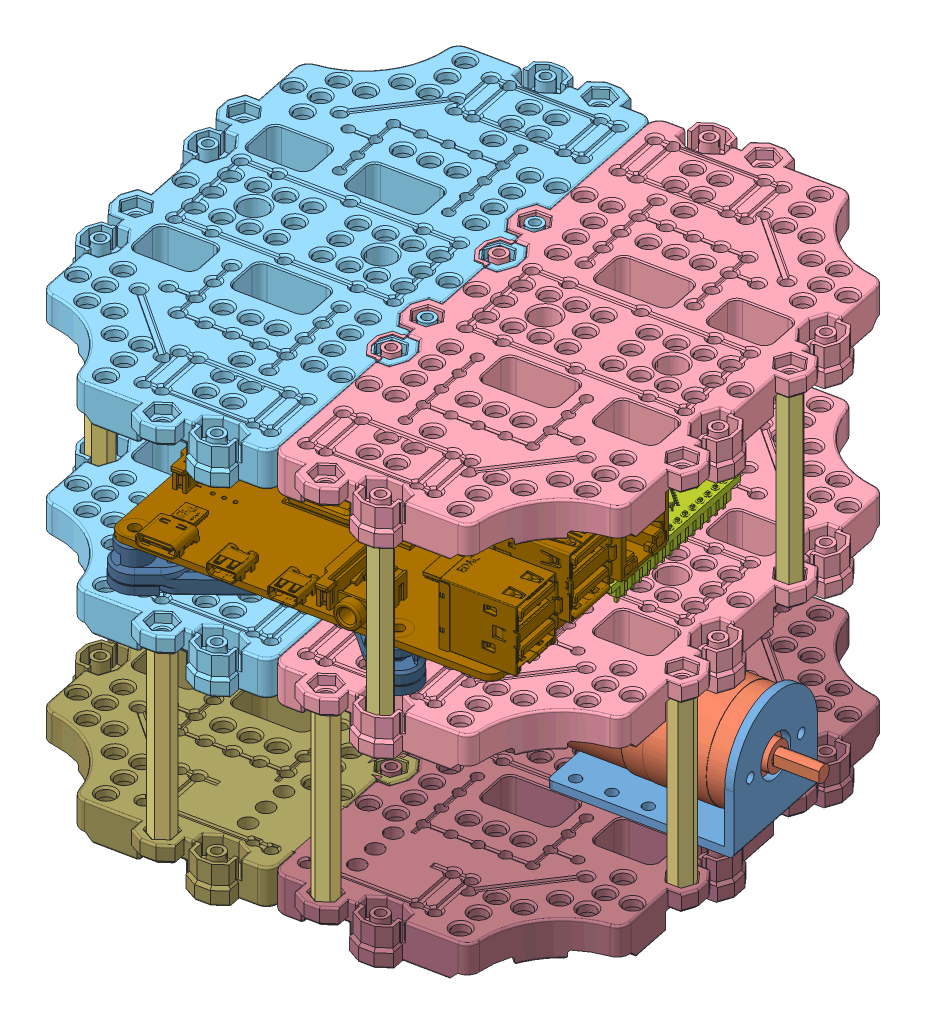
SolidWorks assembly base_link, configuration Default. Lengths in mm.
Overall size (162.47 104.15 162.47).
33 component instances, 13 part files, 91 mates.
Components (placement in the parent):
- motor_support-1: motor_support [Default] at (-43.4369 -3.9762 107.463) x (-0.201684 0 -0.979451) z (0.979451 0 -0.201684) size (28 29 41)
- motor_support-2: motor_support [Default] at (91.2839 -3.9762 79.7219) x (0.201684 0 0.979451) z (-0.979451 0 0.201684) size (28 29 41)
- JGA25-370-1: JGA25-370 [Default] at (46.94 -3.9762 88.853) x (0.979451 0 -0.201684) z (0 -1 0) size (70.5 25.2 25.2)
- JGA25-370-2: JGA25-370 [Default] at (0.907 -3.9762 98.3319) x (-0.979451 0 0.201684) z (0 -1 0) size (70.5 25.2 25.2)
- SUPPORT_HEX_M3_0XL45_FF-1: SUPPORT_HEX_M3_0XL45_FF [Default] at (34.5226 -21.4762 26.0672) x (-0.5 0 0.866025) z (-0.866025 0 -0.5) size (5 45 5.77)
- SUPPORT_HEX_M3_0XL45_FF-6: SUPPORT_HEX_M3_0XL45_FF [Default] at (13.3245 -21.4762 161.1177) x (0.255141 0 -0.966904) z (0.966904 0 0.255141) size (5 45 5.77)
- waffle_front_plate-3: waffle_front_plate [Default] at (23.9235 28.0238 93.5924) x (0.979451 0 -0.201684) z (0.201684 0 0.979451) size (73.55 9.85 137.55)
- waffle_rear_plate-2: waffle_rear_plate [Default] at (23.9235 28.0238 93.5924) x (-0.979451 0 0.201684) z (-0.201684 0 -0.979451) size (73.55 9.85 137.55)
- SUPPORT_HEX_M3_0XL45_FF-7: SUPPORT_HEX_M3_0XL45_FF [Default] at (-12.4911 -23.9762 35.748) x (0 0 -1) z (1 0 0) size (5 45 5.77)
- SUPPORT_HEX_M3_0XL45_FF-17: SUPPORT_HEX_M3_0XL45_FF [Default] at (-43.6018 23.5238 82.9934) x (0.866025 0 0.5) z (0.5 0 -0.866025) size (5 45 5.77)
- SUPPORT_HEX_M3_0XL45_FF-18: SUPPORT_HEX_M3_0XL45_FF [Default] at (91.4488 23.5238 104.1915) x (0.866025 0 0.5) z (0.5 0 -0.866025) size (5 45 5.77)
- L298N-2: L298N [Default] at (1.533 38.0238 65.2768) x (0.979451 0 -0.201684) z (0.201684 0 0.979451) size (50 22 50)
- Arduino Nano-2: Arduino Nano [Default] at (32.4135 30.0238 59.7967) x (0.201684 0 0.979451) z (0 1 0) size (44.28 18 13.68)
- board_bracket_small-1: board_bracket_small [Default] at (19.5539 28.0238 39.0638) x (0.977292 0 -0.211899) z (0.211899 0 0.977292) size (37.82 10 10.43)
- board_bracket_small-2: board_bracket_small [Default] at (-16.4879 28.0238 91.4897) x (0.231228 0 0.9729) z (-0.9729 0 0.231228) size (37.82 10 10.43)
- board_bracket_small-3: board_bracket_small [Default] at (28.444 28.0238 82.2376) x (0.272036 0 0.962287) z (-0.962287 0 0.272036) size (37.82 10 10.43)
- SUPPORT_HEX_M3_0XL45_FF-20: SUPPORT_HEX_M3_0XL45_FF [Default] at (-33.9209 68.3238 130.007) x (0.664389 0 0.747387) z (0.747387 0 -0.664389) size (5 45 5.77)
- SUPPORT_HEX_M3_0XL45_FF-21: SUPPORT_HEX_M3_0XL45_FF [Default] at (-0.7377 70.5238 33.3278) x (-0.979451 0 0.201684) z (0.201684 0 0.979451) size (5 45 5.77)
- SUPPORT_HEX_M3_0XL45_FF-22: SUPPORT_HEX_M3_0XL45_FF [Default] at (-41.1815 68.3238 94.7468) x (-0.315062 0 0.949071) z (0.949071 0 0.315062) size (5 45 5.77)
- SUPPORT_HEX_M3_0XL45_FF-23: SUPPORT_HEX_M3_0XL45_FF [Default] at (22.7691 68.3238 28.4874) x (0.201684 0 0.979451) z (0.979451 0 -0.201684) size (5 45 5.77)
- SUPPORT_HEX_M3_0XL45_FF-25: SUPPORT_HEX_M3_0XL45_FF [Default] at (48.5847 23.5238 153.8571) x (1 0 0) z (0 0 -1) size (5 45 5.77)
- SUPPORT_HEX_M3_0XL45_FF-26: SUPPORT_HEX_M3_0XL45_FF [Default] at (60.3381 68.3238 151.4369) x (0.949071 0 0.315062) z (0.315062 0 -0.949071) size (5 45 5.77)
- SUPPORT_HEX_M3_0XL45_FF-27: SUPPORT_HEX_M3_0XL45_FF [Default] at (84.1881 70.5238 68.9313) x (0.201684 0 0.979451) z (0.979451 0 -0.201684) size (5 45 5.77)
- Raspberry Pi 4 Model B-3: Raspberry Pi 4 Model B [Default] at (147.2874 -46.1762 96.888) x (0.979451 0 -0.201684) z (0 1 0) size (89.07 58.45 20.84)
- board_bracket-5: board_bracket [Default] at (57.1744 28.0238 143.6412) x (0.831623 0 0.555341) z (-0.555341 0 0.831623) size (37.82 10 10.2)
- board_bracket-6: board_bracket [Default] at (47.2919 28.0238 95.6482) x (-0.4133 0 -0.910595) z (0.910595 0 -0.4133) size (37.82 10 10.2)
- board_bracket-7: board_bracket [Default] at (0.3663 28.0238 155.3389) x (-0.712859 0 0.701307) z (-0.701307 0 -0.712859) size (37.82 10 10.2)
- board_bracket-8: board_bracket [Default] at (-9.5162 28.0238 107.3458) x (-0.699696 0 -0.714441) z (0.714441 0 -0.699696) size (37.82 10 10.2)
- waffle_rear_plate-3: waffle_rear_plate [Default] at (23.9235 75.0238 93.5924) x (-0.979451 0 0.201684) z (-0.201684 0 -0.979451) size (73.55 9.85 137.55)
- waffle_front_plate-4: waffle_front_plate [Default] at (23.9235 75.3238 93.5924) x (0.979451 0 -0.201684) z (0.201684 0 0.979451) size (73.55 9.85 137.55)
- MPU_6050-1: MPU_6050 [Default] at (26.3064 64.8238 100.2299) x (1 0 0) z (0 -1 0) size (20.5 16 3)
- waffle_rear_base_plate-1: waffle_rear_base_plate [Default] at (23.9235 -18.9762 93.5924) x (-0.979451 0 0.201684) z (-0.201684 0 -0.979451) size (73.55 9.85 137.55)
- waffle_front_base_plate-1: waffle_front_base_plate [Default] at (23.9235 -18.9762 93.5924) x (0.979451 0 -0.201684) z (0.201684 0 0.979451) size (73.55 9.85 137.55)
Mates (geometry in assembly coordinates):
- Coincident21: coincident anti-aligned: plane of motor_support-2 through (89.325 -3.9762 80.1253) normal (-0.979451 0 0.201684); plane of JGA25-370-1 through (91.846 -3.9762 92.3684) normal (0.979451 0 -0.201684)
- Concentric7: concentric aligned: circle of motor_support-2; circle of JGA25-370-1
- Concentric8: concentric aligned: cylinder of motor_support-2 through (87.6107 -3.9762 71.8) axis (0.979451 0 -0.201684) radius 1.25; cylinder of JGA25-370-1 through (82.7134 -3.9762 72.8084) axis (0.979451 0 -0.201684) radius 1.25
- Coincident22: coincident anti-aligned: plane of motor_support-1 through (-41.478 -3.9762 107.0596) normal (0.979451 0 -0.201684); plane of JGA25-370-2 through (-43.999 -3.9762 94.8165) normal (-0.979451 0 0.201684)
- Concentric9: concentric aligned: circle of motor_support-1; circle of JGA25-370-2
- Concentric10: concentric anti-aligned: circle of motor_support-1; circle of JGA25-370-2
- Coincident72: coincident anti-aligned: plane of SUPPORT_HEX_M3_0XL45_FF-1 through (34.5226 23.5238 26.0672) normal (0 1 0); plane of waffle_front_plate-3 through (23.9235 23.5238 93.5924) normal (0 -1 0)
- Concentric28: concentric anti-aligned: cylinder of SUPPORT_HEX_M3_0XL45_FF-1 through (34.5226 12.2352 26.0672) axis (0 -1 0) radius 1.25; cylinder of waffle_front_plate-3 through (34.5226 17.6288 26.0672) axis (0 1 0) radius 1.6
- Concentric30: concentric anti-aligned: cylinder of SUPPORT_HEX_M3_0XL45_FF-6 through (13.3245 12.2352 161.1177) axis (0 -1 0) radius 1.25; cylinder of waffle_rear_plate-2 through (13.3245 17.6288 161.1177) axis (0 1 0) radius 1.6
- Coincident74: coincident anti-aligned: plane of SUPPORT_HEX_M3_0XL45_FF-6 through (13.3245 23.5238 161.1177) normal (0 1 0); plane of waffle_rear_plate-2 through (23.9235 23.5238 93.5924) normal (0 -1 0)
- Concentric33: concentric aligned: circle of waffle_rear_plate-2; circle of SUPPORT_HEX_M3_0XL45_FF-7
- Parallel33: parallel aligned: plane of waffle_rear_plate-2 through (-1.7004 25.7738 28.6524) normal (-0.201684 0 -0.979451); plane of L298N-2 through (-27.9954 39.0238 45.8326) normal (-0.201684 0 -0.979451)
- Parallel34: parallel anti-aligned: plane of waffle_front_plate-3 through (23.9235 28.0238 93.5924) normal (0 1 0); plane of L298N-2 through (1.533 38.0238 65.2768) normal (0 -1 0)
- Parallel35: parallel aligned: plane of waffle_front_plate-3 through (73.7006 28.0238 17.9998) normal (-0.201684 0 -0.979451); plane of Arduino Nano-2 through (61.4124 34.1638 58.9763) normal (-0.201684 0 -0.979451)
- Parallel36: parallel anti-aligned: plane of waffle_front_plate-3 through (23.9235 28.0238 93.5924) normal (0 1 0); plane of Arduino Nano-2 through (45.9023 32.5638 66.06) normal (0 -1 0)
- Concentric72: concentric aligned: cylinder of L298N-2 through (19.5539 38.0238 39.0638) axis (0 1 0) radius 1.5; circle of board_bracket_small-1
- Coincident123: coincident anti-aligned: plane of L298N-2 through (1.533 38.0238 65.2768) normal (0 -1 0); plane of board_bracket_small-1 through (19.5539 38.0238 39.0638) normal (0 1 0)
- Coincident124: coincident anti-aligned: plane of waffle_rear_plate-2 through (23.9235 28.0238 93.5924) normal (0 1 0); plane of board_bracket_small-1 through (-7.5359 28.0238 44.9375) normal (0 -1 0)
- Concentric73: concentric anti-aligned: cylinder of waffle_rear_plate-2 through (-7.5359 28.0238 44.9375) axis (0 -1 0) radius 2.5; cylinder of board_bracket_small-1 through (-7.5359 14.9878 44.9375) axis (0 1 0) radius 5
- Lock5: lock: unknown of waffle_front_plate-3; unknown of board_bracket_small-1
- Concentric75: concentric aligned: circle of L298N-2; cylinder of board_bracket_small-2 through (-16.4879 38.0238 91.4897) axis (0 1 0) radius 1
- Coincident125: coincident anti-aligned: plane of L298N-2 through (1.533 38.0238 65.2768) normal (0 -1 0); plane of board_bracket_small-2 through (-16.4879 38.0238 91.4897) normal (0 1 0)
- Lock6: lock: unknown of waffle_rear_plate-2; unknown of board_bracket_small-2
- Concentric78: concentric aligned: cylinder of L298N-2 through (28.444 38.0238 82.2376) axis (0 1 0) radius 1.5; cylinder of board_bracket_small-3 through (28.444 38.0238 82.2376) axis (0 1 0) radius 1
- Coincident126: coincident anti-aligned: plane of L298N-2 through (1.533 38.0238 65.2768) normal (0 -1 0); plane of board_bracket_small-3 through (28.444 38.0238 82.2376) normal (0 1 0)
- Lock7: lock: unknown of waffle_front_plate-3; unknown of board_bracket_small-3
- Concentric81: concentric aligned: circle of waffle_rear_plate-2; cylinder of SUPPORT_HEX_M3_0XL45_FF-20 through (-33.9209 34.6124 130.007) axis (0 1 0) radius 1.25
- Coincident129: coincident anti-aligned: plane of waffle_rear_plate-2 through (23.9235 23.3238 93.5924) normal (0 1 0); plane of SUPPORT_HEX_M3_0XL45_FF-20 through (-33.9209 23.3238 130.007) normal (0 -1 0)
- Parallel44: parallel aligned: plane of waffle_rear_plate-2 through (-38.3256 28.0238 129.3098) normal (-0.979451 0 0.201684); plane of SUPPORT_HEX_M3_0XL45_FF-20 through (-36.0784 68.3238 131.925) normal (-0.979451 0 0.201684)
- Concentric82: concentric aligned: cylinder of waffle_rear_plate-2 through (-0.7377 17.6288 33.3278) axis (0 1 0) radius 1.6; cylinder of SUPPORT_HEX_M3_0XL45_FF-21 through (-0.7377 36.8124 33.3278) axis (0 1 0) radius 1.25
- Coincident131: coincident anti-aligned: plane of waffle_rear_plate-2 through (23.9235 25.5238 93.5924) normal (0 1 0); plane of SUPPORT_HEX_M3_0XL45_FF-21 through (-0.7377 25.5238 33.3278) normal (0 -1 0)
- Concentric83: concentric anti-aligned: cylinder of waffle_rear_plate-2 through (-41.1815 28.0238 94.7468) axis (0 1 0) radius 1.2; circle of SUPPORT_HEX_M3_0XL45_FF-22
- Coincident133: coincident anti-aligned: plane of waffle_rear_plate-2 through (23.9235 23.3238 93.5924) normal (0 1 0); plane of SUPPORT_HEX_M3_0XL45_FF-22 through (-41.1815 23.3238 94.7468) normal (0 -1 0)
- Parallel46: parallel aligned: plane of waffle_rear_plate-2 through (-45.5862 28.0238 94.0495) normal (-0.979451 0 0.201684); plane of SUPPORT_HEX_M3_0XL45_FF-22 through (-43.3391 68.3238 96.6647) normal (-0.979451 0 0.201684)
- Concentric84: concentric aligned: cylinder of waffle_front_plate-3 through (22.7691 28.0238 28.4874) axis (0 1 0) radius 1.2; cylinder of SUPPORT_HEX_M3_0XL45_FF-23 through (22.7691 34.6124 28.4874) axis (0 1 0) radius 1.25
- Coincident135: coincident anti-aligned: plane of waffle_front_plate-3 through (23.9235 23.3238 93.5924) normal (0 1 0); plane of SUPPORT_HEX_M3_0XL45_FF-23 through (22.7691 23.3238 28.4874) normal (0 -1 0)
- Parallel47: parallel aligned: plane of waffle_front_plate-3 through (23.4664 28.0238 24.0828) normal (-0.201684 0 -0.979451); plane of SUPPORT_HEX_M3_0XL45_FF-23 through (20.8512 68.3238 26.3299) normal (-0.201684 0 -0.979451)
- Concentric87: concentric aligned: cylinder of waffle_front_plate-3 through (60.3381 28.0238 151.4369) axis (0 1 0) radius 1.2; cylinder of SUPPORT_HEX_M3_0XL45_FF-26 through (60.3381 34.6124 151.4369) axis (0 1 0) radius 1.25
- Coincident141: coincident anti-aligned: plane of waffle_front_plate-3 through (23.9235 23.3238 93.5924) normal (0 1 0); plane of SUPPORT_HEX_M3_0XL45_FF-26 through (60.3381 23.3238 151.4369) normal (0 -1 0)
- Parallel50: parallel aligned: plane of waffle_front_plate-3 through (59.6408 28.0238 155.8415) normal (0.201684 0 0.979451); plane of SUPPORT_HEX_M3_0XL45_FF-26 through (62.256 68.3238 153.5944) normal (0.201684 0 0.979451)
- Concentric88: concentric aligned: circle of waffle_front_plate-3; cylinder of SUPPORT_HEX_M3_0XL45_FF-27 through (84.1881 36.8124 68.9313) axis (0 1 0) radius 1.25
- Coincident143: coincident anti-aligned: plane of waffle_front_plate-3 through (23.9235 25.5238 93.5924) normal (0 1 0); plane of SUPPORT_HEX_M3_0XL45_FF-27 through (84.1881 25.5238 68.9313) normal (0 -1 0)
- Parallel51: parallel aligned: plane of waffle_front_plate-3 through (88.024 28.0238 73.2463) normal (0.949071 0 0.315062); plane of SUPPORT_HEX_M3_0XL45_FF-27 through (87.0156 70.5238 68.3491) normal (0.949071 0 0.315062)
- Parallel52: parallel anti-aligned: plane of waffle_rear_plate-2 through (23.9235 28.0238 93.5924) normal (0 1 0); plane of Raspberry Pi 4 Model B-3 through (-0.0226 38.0238 155.9295) normal (0 -1 0)
- Parallel53: parallel aligned: plane of waffle_front_plate-3 through (36.8313 28.0238 156.2773) normal (0.201684 0 0.979451); plane of Raspberry Pi 4 Model B-3 through (0.5825 39.6238 158.8678) normal (0.201684 0 0.979451)
- Parallel54: parallel aligned: plane of waffle_front_plate-3 through (99.5161 28.0238 143.3695) normal (0.979451 0 -0.201684); plane of Raspberry Pi 4 Model B-3 through (80.2924 39.6238 139.3914) normal (0.979451 0 -0.201684)
- Coincident148: coincident aligned: plane of waffle_front_plate-3 through (59.3753 25.7738 146.7615) normal (0.201684 0 0.979451); plane of Raspberry Pi 4 Model B-3 through (0.5825 39.6238 158.8678) normal (0.201684 0 0.979451)
- Concentric90: concentric anti-aligned: cylinder of Raspberry Pi 4 Model B-3 through (57.1744 37.9238 143.6412) axis (0 1 0) radius 1.35; cylinder of board_bracket-5 through (57.1744 39.0238 143.6412) axis (0 -1 0) radius 2
- Coincident149: coincident anti-aligned: plane of Raspberry Pi 4 Model B-3 through (-0.0226 38.0238 155.9295) normal (0 -1 0); plane of board_bracket-5 through (50.2396 38.0238 145.0227) normal (0 1 0)
- Coincident150: coincident anti-aligned: plane of waffle_front_plate-3 through (23.9235 28.0238 93.5924) normal (0 1 0); plane of board_bracket-5 through (51.9029 28.0238 146.1333) normal (0 -1 0)
- Concentric91: concentric aligned: cylinder of waffle_front_plate-3 through (34.1225 27.2238 128.2476) axis (0 1 0) radius 2; cylinder of board_bracket-5 through (34.1225 14.9878 128.2476) axis (0 1 0) radius 5
- Concentric92: concentric anti-aligned: cylinder of Raspberry Pi 4 Model B-3 through (47.2919 37.9238 95.6482) axis (0 1 0) radius 1.35; cylinder of board_bracket-6 through (47.2919 39.0238 95.6482) axis (0 -1 0) radius 2
- Coincident151: coincident anti-aligned: plane of Raspberry Pi 4 Model B-3 through (-0.0226 38.0238 155.9295) normal (0 -1 0); plane of board_bracket-6 through (53.9114 38.0238 98.1346) normal (0 1 0)
- Lock8: lock: unknown of waffle_front_plate-3; unknown of board_bracket-6
- Concentric94: concentric anti-aligned: cylinder of Raspberry Pi 4 Model B-3 through (0.3663 37.9238 155.3389) axis (0 1 0) radius 1.35; cylinder of board_bracket-7 through (0.3663 39.0238 155.3389) axis (0 -1 0) radius 2
- Coincident152: coincident anti-aligned: plane of Raspberry Pi 4 Model B-3 through (-0.0226 38.0238 155.9295) normal (0 -1 0); plane of board_bracket-7 through (0.4241 38.0238 148.2681) normal (0 1 0)
- Lock9: lock: unknown of waffle_rear_plate-2; unknown of board_bracket-7
- Concentric96: concentric anti-aligned: cylinder of Raspberry Pi 4 Model B-3 through (-9.5162 37.9238 107.3458) axis (0 1 0) radius 1.3; cylinder of board_bracket-8 through (-9.5162 39.0238 107.3458) axis (0 -1 0) radius 2
- Coincident153: coincident anti-aligned: plane of Raspberry Pi 4 Model B-3 through (-0.0226 38.0238 155.9295) normal (0 -1 0); plane of board_bracket-8 through (-2.4455 38.0238 107.4195) normal (0 1 0)
- Lock10: lock: unknown of waffle_rear_plate-2; unknown of board_bracket-8
- Parallel58: parallel anti-aligned: plane of waffle_rear_plate-2 through (1.6788 28.0238 31.1797) normal (-0.315062 0 0.949071); plane of SUPPORT_HEX_M3_0XL45_FF-21 through (-1.3199 70.5238 30.5004) normal (0.315062 0 -0.949071)
- Concentric98: concentric aligned: cylinder of SUPPORT_HEX_M3_0XL45_FF-21 through (-0.7377 59.2352 33.3278) axis (0 1 0) radius 1.25; cylinder of waffle_rear_plate-3 through (-0.7377 64.6288 33.3278) axis (0 1 0) radius 1.6
- Coincident156: coincident anti-aligned: plane of SUPPORT_HEX_M3_0XL45_FF-21 through (-0.7377 70.5238 33.3278) normal (0 1 0); plane of waffle_rear_plate-3 through (23.9235 70.5238 93.5924) normal (0 -1 0)
- Concentric99: concentric aligned: cylinder of SUPPORT_HEX_M3_0XL45_FF-20 through (-33.9209 57.0352 130.007) axis (0 1 0) radius 1.25; cylinder of waffle_rear_plate-3 through (-33.9209 75.0238 130.007) axis (0 1 0) radius 1.2
- Concentric100: concentric aligned: cylinder of SUPPORT_HEX_M3_0XL45_FF-23 through (22.7691 57.0352 28.4874) axis (0 1 0) radius 1.25; cylinder of waffle_front_plate-4 through (22.7691 64.9288 28.4874) axis (0 1 0) radius 1.6
- Coincident157: coincident anti-aligned: plane of SUPPORT_HEX_M3_0XL45_FF-23 through (22.7691 68.3238 28.4874) normal (0 1 0); plane of waffle_front_plate-4 through (23.9235 68.3238 93.5924) normal (0 -1 0)
- Concentric101: concentric aligned: cylinder of SUPPORT_HEX_M3_0XL45_FF-26 through (60.3381 57.0352 151.4369) axis (0 1 0) radius 1.25; cylinder of waffle_front_plate-4 through (60.3381 75.3238 151.4369) axis (0 1 0) radius 1.2
- Coincident173: coincident anti-aligned: plane of waffle_front_plate-4 through (23.9235 66.3238 93.5924) normal (0 -1 0); plane of MPU_6050-1 through (26.3064 66.3238 100.2299) normal (0 1 0)
- Concentric119: concentric aligned: circle of waffle_rear_plate-3; cylinder of MPU_6050-1 through (18.3064 64.8238 105.9799) axis (0 1 0) radius 1.5
- Concentric122: concentric anti-aligned: cylinder of waffle_front_plate-3 through (48.5847 17.6288 153.8571) axis (0 1 0) radius 1.6; circle of SUPPORT_HEX_M3_0XL45_FF-25
- Concentric124: concentric anti-aligned: cylinder of SUPPORT_HEX_M3_0XL45_FF-6 through (13.3245 -10.1876 161.1177) axis (0 -1 0) radius 1.25; cylinder of waffle_rear_base_plate-1 through (13.3245 -29.3712 161.1177) axis (0 1 0) radius 1.6
- Coincident178: coincident anti-aligned: plane of SUPPORT_HEX_M3_0XL45_FF-6 through (13.3245 -21.4762 161.1177) normal (0 -1 0); plane of waffle_rear_base_plate-1 through (23.9235 -21.4762 93.5924) normal (0 1 0)
- Concentric125: concentric anti-aligned: cylinder of SUPPORT_HEX_M3_0XL45_FF-7 through (-12.4911 -12.6876 35.748) axis (0 -1 0) radius 1.25; cylinder of waffle_rear_base_plate-1 through (-12.4911 -18.9762 35.748) axis (0 1 0) radius 1.2
- Coincident179: coincident anti-aligned: plane of motor_support-1 through (-44.3015 -18.9762 93.3473) normal (0 -1 0); plane of waffle_rear_base_plate-1 through (23.9235 -18.9762 93.5924) normal (0 1 0)
- Coincident180: coincident anti-aligned: circle of motor_support-1; cylinder of waffle_rear_base_plate-1 through (-5.2004 -27.9762 110.8203) axis (0 -1 0) radius 1.35
- Concentric126: concentric anti-aligned: cylinder of motor_support-1 through (-33.1443 -33.9762 94.1128) axis (0 1 0) radius 1.35; cylinder of waffle_rear_base_plate-1 through (-33.1443 -27.9762 94.1128) axis (0 -1 0) radius 1.35
- Coincident181: coincident anti-aligned: plane of waffle_front_plate-3 through (23.9235 23.5238 93.5924) normal (0 -1 0); plane of SUPPORT_HEX_M3_0XL45_FF-25 through (48.5847 23.5238 153.8571) normal (0 1 0)
- Coincident182: coincident anti-aligned: plane of waffle_front_plate-3 through (23.9235 23.5238 93.5924) normal (0 -1 0); plane of SUPPORT_HEX_M3_0XL45_FF-18 through (91.4488 23.5238 104.1915) normal (0 1 0)
- Coincident184: coincident anti-aligned: plane of waffle_rear_plate-2 through (23.9235 21.0238 93.5924) normal (0 -1 0); plane of SUPPORT_HEX_M3_0XL45_FF-7 through (-12.4911 21.0238 35.748) normal (0 1 0)
- Coincident185: coincident anti-aligned: plane of waffle_rear_plate-2 through (23.9235 23.5238 93.5924) normal (0 -1 0); plane of SUPPORT_HEX_M3_0XL45_FF-17 through (-43.6018 23.5238 82.9934) normal (0 1 0)
- Concentric127: concentric anti-aligned: cylinder of waffle_front_plate-3 through (91.4488 17.6288 104.1915) axis (0 1 0) radius 1.6; circle of SUPPORT_HEX_M3_0XL45_FF-18
- Concentric128: concentric anti-aligned: circle of waffle_rear_plate-2; cylinder of SUPPORT_HEX_M3_0XL45_FF-17 through (-43.6018 12.2352 82.9934) axis (0 1 0) radius 1.25
- Concentric129: concentric aligned: cylinder of SUPPORT_HEX_M3_0XL45_FF-17 through (-43.6018 12.2352 82.9934) axis (0 1 0) radius 1.25; cylinder of waffle_rear_base_plate-1 through (-43.6018 -29.3712 82.9934) axis (0 1 0) radius 1.6
- Coincident186: coincident anti-aligned: plane of waffle_front_plate-3 through (23.9235 28.0238 93.5924) normal (0 1 0); plane of Arduino Nano-2 through (45.9023 28.0238 66.06) normal (0 -1 0)
- Coincident187: coincident aligned: plane of waffle_front_plate-3 through (61.8851 28.0238 61.272) normal (0.979451 0 -0.201684); plane of Arduino Nano-2 through (61.4124 34.1638 58.9763) normal (0.979451 0 -0.201684)
- Concentric130: concentric anti-aligned: circle of waffle_rear_base_plate-1; cylinder of waffle_front_base_plate-1 through (28.7639 -18.9762 117.0993) axis (0 1 0) radius 1.2
- Concentric131: concentric aligned: cylinder of waffle_rear_base_plate-1 through (19.0831 -18.9762 70.0856) axis (0 1 0) radius 1.2; cylinder of waffle_front_base_plate-1 through (19.0831 -29.3712 70.0856) axis (0 1 0) radius 1.6
- Coincident189: coincident aligned: plane of waffle_rear_base_plate-1 through (22.9703 -22.9762 148.4622) normal (0 -1 0); plane of waffle_front_base_plate-1 through (46.4771 -22.9762 143.6218) normal (0 -1 0)
- Coincident190: coincident anti-aligned: plane of motor_support-2 through (92.1486 -18.9762 93.8376) normal (0 -1 0); plane of waffle_front_base_plate-1 through (23.9235 -18.9762 93.5924) normal (0 1 0)
- Concentric132: concentric anti-aligned: cylinder of motor_support-2 through (57.4844 -33.9762 97.9125) axis (0 1 0) radius 1.35; cylinder of waffle_front_base_plate-1 through (57.4844 -27.9762 97.9125) axis (0 -1 0) radius 1.35
- Concentric133: concentric anti-aligned: cylinder of motor_support-2 through (76.5542 -33.9762 71.5242) axis (0 1 0) radius 1.35; cylinder of waffle_front_base_plate-1 through (76.5542 -27.9762 71.5242) axis (0 -1 0) radius 1.35
